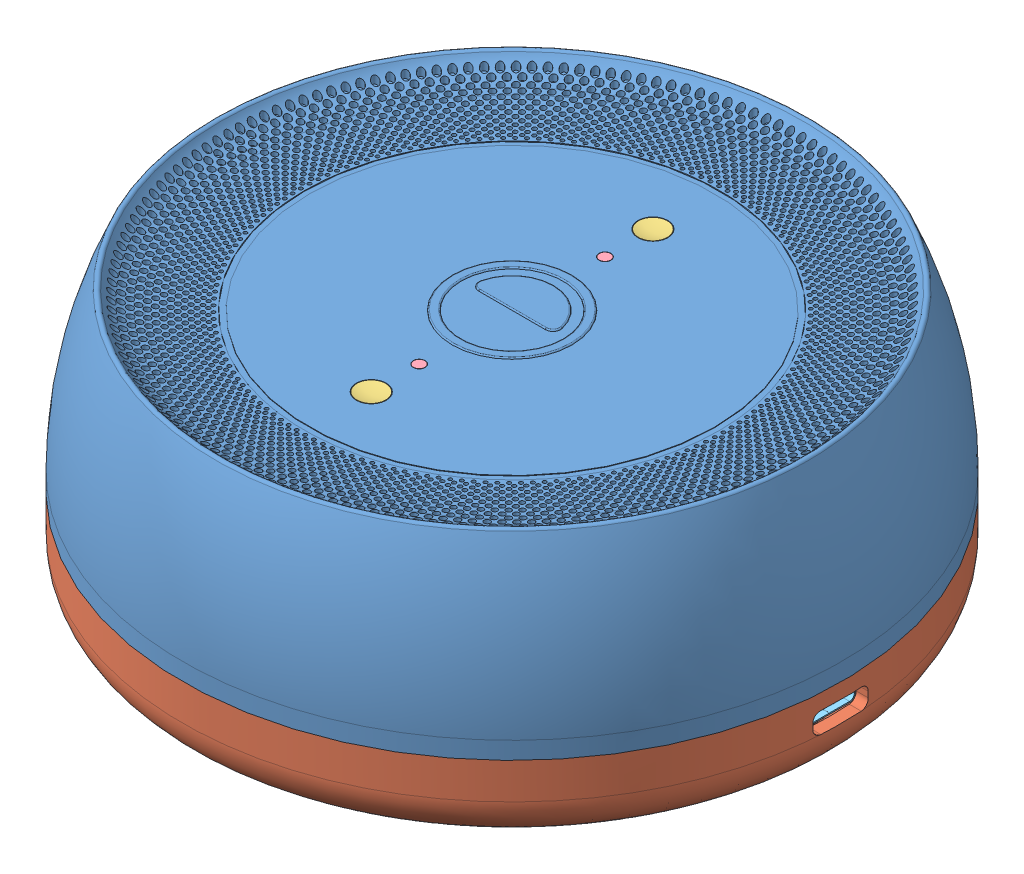
SolidWorks assembly Сборка, configuration Default. Lengths in mm.
Overall size (110 43.02 110).
434 component instances, 58 part files, 28 mates.
Components (placement in the parent):
- Корпус-1: Корпус [Default] at (55.5185 45.3642 75.701) size (110 29.48 110)
- Крышка-1: Крышка [Default] at (55.5185 43.2142 75.701) size (110 20.5 110)
- Кнопка-1: Кнопка [Default] at (55.5185 66.8642 99.201) size (7 2.5 7)
- Кнопка-2: Кнопка [Default] at (55.5185 66.8642 52.201) size (7 2.5 7)
- Держатель батареек-1: Держатель батареек [Default] at (94.5185 37.2764 95.701) x (0 0 -1) z (1 0 0) size (40 21.5 78)
- ME2CO-1: ME2CO [Default] at (52.3216 36.0894 105.6741) size (20 17 20)
- bottom_test_pcb-2: bottom_test_pcb [Default] at (55.5185 35.6764 75.701) x (1 0 0) z (0 -1 0) size (102.89 89.9 16)
  - USB Type C-1: USB Type C [По умолчанию] at origin size (11.79 8.75 4.86)
    - 632723300011-1: 632723300011 [По умолчанию] at (48.1249 -0.0001 -3.2614) x (0 1 0) z (1 0 0) size (8.75 4.86 11.79)
      - 632723300011_Shielding_2-1: 632723300011_Shielding_2 [По умолчанию] at (0 -0.8 -1.425) x (0 0 1) z (0 -1 0) size (2.92 7.5 1.07)
      - 632723300011_Shielding_2-2: 632723300011_Shielding_2 [По умолчанию] at (0 0.75 -1.425) x (0 0 1) z (0 1 0) size (2.92 7.5 1.07)
      - 632723300011_Housing_Bottom3-1: 632723300011_Housing_Bottom3 [По умолчанию] at (0 0.89 -5.284) x (-1 0 0) z (0 -1 0) size (6.46 2.1 0.78)
      - 632723300011_PIN7_Bottom_v3_mir-1: 632723300011_PIN7_Bottom_v3_mir [По умолчанию] at (0.4 3.3765 -5.46) x (-1 0 0) z (0 -1 0) size (0.54 7.67 3.25)
      - 632723300011_PIN5_Bottom_v3_mir-1: 632723300011_PIN5_Bottom_v3_mir [По умолчанию] at (1.2 3.3765 -5.46) x (-1 0 0) z (0 -1 0) size (0.37 8.17 3.21)
      - 632723300011_PIN2_Bottom_v3_mir-1: 632723300011_PIN2_Bottom_v3_mir [По умолчанию] at (2.4 3.3765 -4.75) x (-1 0 0) z (0 -1 0) size (0.54 6.96 3.25)
      - 632723300011_PIN6_Bottom_v3_mir-1: 632723300011_PIN6_Bottom_v3_mir [По умолчанию] at (0.8 3.3765 -4.76) x (-1 0 0) z (0 -1 0) size (0.4 6.97 3.21)
      - 632723300011_PIN4_Bottom_v3_mir-1: 632723300011_PIN4_Bottom_v3_mir [По умолчанию] at (1.6 3.3765 -4.7565) x (-1 0 0) z (0 -1 0) size (0.52 7.01 3.21)
      - 632723300011_PIN1_Bottom_v3_mir-1: 632723300011_PIN1_Bottom_v3_mir [По умолчанию] at (2.8 3.3765 -5.46) x (-1 0 0) z (0 -1 0) size (0.4 8.17 3.21)
      - 632723300011_PIN2_Top_v3-1: 632723300011_PIN2_Top_v3 [По умолчанию] at (1.75 2.37 -6.335) x (0 0 1) z (0 -1 0) size (9.09 0.28 1.93)
      - 632723300011_PIN2_Top_v3-2: 632723300011_PIN2_Top_v3 [По умолчанию] at (-1.75 2.37 -6.335) x (0 0 1) z (0 -1 0) size (9.09 0.28 1.93)
      - 632723300011_PIN2_Top_v3-3: 632723300011_PIN2_Top_v3 [По умолчанию] at (-0.75 2.37 -6.335) x (0 0 1) z (0 -1 0) size (9.09 0.28 1.93)
      - 632723300011_PIN2_Top_v3-4: 632723300011_PIN2_Top_v3 [По умолчанию] at (0.75 2.37 -6.335) x (0 0 1) z (0 -1 0) size (9.09 0.28 1.93)
      - 632723300011_PIN2_Top_v3-5: 632723300011_PIN2_Top_v3 [По умолчанию] at (-0.25 2.37 -6.335) x (0 0 1) z (0 -1 0) size (9.09 0.28 1.93)
      - 632723300011_PIN2_Top_v3-6: 632723300011_PIN2_Top_v3 [По умолчанию] at (2.25 2.37 -6.335) x (0 0 1) z (0 -1 0) size (9.09 0.28 1.93)
      - 632723300011_PIN2_Top_v3-7: 632723300011_PIN2_Top_v3 [По умолчанию] at (0.25 2.37 -6.335) x (0 0 1) z (0 -1 0) size (9.09 0.28 1.93)
      - 632723300011_PIN2_Top_v3-8: 632723300011_PIN2_Top_v3 [По умолчанию] at (-2.25 2.37 -6.335) x (0 0 1) z (0 -1 0) size (9.09 0.28 1.93)
      - 632723300011_PIN7_Bottom_v3-1: 632723300011_PIN7_Bottom_v3 [По умолчанию] at (-0.4 3.3765 -5.46) x (1 0 0) z (0 -1 0) size (0.54 7.67 3.21)
      - 632723300011_PIN6_Bottom_v3-1: 632723300011_PIN6_Bottom_v3 [По умолчанию] at (-0.8 3.3765 -4.76) x (1 0 0) z (0 -1 0) size (0.4 6.97 3.22)
      - 632723300011_PIN5_Bottom_v3-1: 632723300011_PIN5_Bottom_v3 [По умолчанию] at (-1.2 3.3765 -5.46) x (1 0 0) z (0 -1 0) size (0.37 8.17 3.19)
      - 632723300011_PIN4_Bottom_v3-1: 632723300011_PIN4_Bottom_v3 [По умолчанию] at (-1.6 3.3765 -4.7565) x (1 0 0) z (0 -1 0) size (0.54 7.01 3.25)
      - 632723300011_PIN2_Bottom_v3-1: 632723300011_PIN2_Bottom_v3 [По умолчанию] at (-2.4 3.3765 -4.75) x (1 0 0) z (0 -1 0) size (0.54 6.96 3.21)
      - 632723300011_PIN1_Top_v3-1: 632723300011_PIN1_Top_v3 [По умолчанию] at (2.75 1.97 -6.335) x (0 0 1) z (0 -1 0) size (9.59 0.28 1.93)
      - 632723300011_PIN1_Top_v3-2: 632723300011_PIN1_Top_v3 [По умолчанию] at (-1.25 1.97 -6.335) x (0 0 1) z (0 -1 0) size (9.59 0.28 1.93)
      - 632723300011_PIN1_Top_v3-3: 632723300011_PIN1_Top_v3 [По умолчанию] at (-2.75 1.97 -6.335) x (0 0 1) z (0 -1 0) size (9.59 0.28 1.93)
      - 632723300011_PIN1_Top_v3-4: 632723300011_PIN1_Top_v3 [По умолчанию] at (1.25 1.97 -6.335) x (0 0 1) z (0 -1 0) size (9.59 0.28 1.93)
      - 632723300011_PIN1_Bottom_v3-1: 632723300011_PIN1_Bottom_v3 [По умолчанию] at (-2.8 3.3765 -5.46) x (1 0 0) z (0 -1 0) size (0.4 8.17 3.22)
      - 632723300011_Housing_Bottom-1: 632723300011_Housing_Bottom [По умолчанию] at (0 0.89 -5.285) x (-1 0 0) z (0 -1 0) size (8.34 5.47 2.38)
      - 632723300011_Shielding_1_v3-1: 632723300011_Shielding_1_v3 [По умолчанию] at (0 0 -0.475) x (-1 0 0) z (0 -1 0) size (8.75 10.6 4.86)
      - 632723300011_Housing_TOP-1: 632723300011_Housing_TOP [По умолчанию] at (0 -0.6 -3.9) x (1 0 0) z (0 -1 0) size (6.7 3.25 1.23)
      - 632723300011_Shielding_3_v3-1: 632723300011_Shielding_3_v3 [По умолчанию] at (0 0.05 0) size (7.5 3.43 8.64)
      - 632723300011_Housing-1: 632723300011_Housing [По умолчанию] at origin size (8.34 2.56 8.2)
  - C1-1: C1 [По умолчанию] at origin size (1.8 3.4 1.8)
    - 6038255504-1: 6038255504 [По умолчанию] at (35.6 7.5 0) size (1.8 3.4 1.8)
      - Extruded-1: Extruded [По умолчанию] at origin size (1.8 3.4 1.8)
  - C2-1: C2 [По умолчанию] at origin size (1.45 2.2 1.55)
    - 6038248944-1: 6038248944 [По умолчанию] at (33 7.375 0) size (1.45 0.5 1.55)
      - Extruded-1-1: Extruded-1 [По умолчанию] at origin size (1.45 0.5 1.55)
    - 6038248944-2: 6038248944 [По умолчанию] at (33 5.675 0) size (1.45 0.5 1.55)
      - Extruded-1-1: Extruded-1 [По умолчанию] at origin size (1.45 0.5 1.55)
    - 6038249184-1: 6038249184 [По умолчанию] at (33 6.525 0) size (1.45 1.2 1.55)
      - Extruded-2-1: Extruded-2 [По умолчанию] at origin size (1.45 1.2 1.55)
  - C3-1: C3 [По умолчанию] at origin size (2.2 1.45 1.55)
    - 6038256064-1: 6038256064 [По умолчанию] at (30.15 2.5 0) size (0.5 1.45 1.55)
      - Extruded-3-1: Extruded-3 [По умолчанию] at origin size (0.5 1.45 1.55)
    - 6038256064-2: 6038256064 [По умолчанию] at (28.45 2.5 0) size (0.5 1.45 1.55)
      - Extruded-3-1: Extruded-3 [По умолчанию] at origin size (0.5 1.45 1.55)
    - 6038256544-1: 6038256544 [По умолчанию] at (29.3 2.5 0) size (1.2 1.45 1.55)
      - Extruded-4-1: Extruded-4 [По умолчанию] at origin size (1.2 1.45 1.55)
  - C4-1: C4 [По умолчанию] at origin size (2.2 1.45 1.55)
    - 6038256064-1: 6038256064 [По умолчанию] at (31.95 9.3 0) size (0.5 1.45 1.55)
      - Extruded-3-1: Extruded-3 [По умолчанию] at origin size (0.5 1.45 1.55)
    - 6038256064-2: 6038256064 [По умолчанию] at (30.25 9.3 0) size (0.5 1.45 1.55)
      - Extruded-3-1: Extruded-3 [По умолчанию] at origin size (0.5 1.45 1.55)
    - 6038256544-1: 6038256544 [По умолчанию] at (31.1 9.3 0) size (1.2 1.45 1.55)
      - Extruded-4-1: Extruded-4 [По умолчанию] at origin size (1.2 1.45 1.55)
  - C5-1: C5 [По умолчанию] at origin size (1.8 3.4 1.8)
    - 6038255504-1: 6038255504 [По умолчанию] at (36.9 15.75 0) size (1.8 3.4 1.8)
      - Extruded-1: Extruded [По умолчанию] at origin size (1.8 3.4 1.8)
  - C6-1: C6 [По умолчанию] at origin size (1.45 2.2 1.55)
    - 6038248944-1: 6038248944 [По умолчанию] at (-24.655 -38.95 0) size (1.45 0.5 1.55)
      - Extruded-1-1: Extruded-1 [По умолчанию] at origin size (1.45 0.5 1.55)
    - 6038248944-2: 6038248944 [По умолчанию] at (-24.655 -37.25 0) size (1.45 0.5 1.55)
      - Extruded-1-1: Extruded-1 [По умолчанию] at origin size (1.45 0.5 1.55)
    - 6038249184-1: 6038249184 [По умолчанию] at (-24.655 -38.1 0) size (1.45 1.2 1.55)
      - Extruded-2-1: Extruded-2 [По умолчанию] at origin size (1.45 1.2 1.55)
  - C7-1: C7 [По умолчанию] at origin size (2.2 1.45 1.55)
    - 6038256064-1: 6038256064 [По умолчанию] at (32.8 28.7 0) size (0.5 1.45 1.55)
      - Extruded-3-1: Extruded-3 [По умолчанию] at origin size (0.5 1.45 1.55)
    - 6038256064-2: 6038256064 [По умолчанию] at (34.5 28.7 0) size (0.5 1.45 1.55)
      - Extruded-3-1: Extruded-3 [По умолчанию] at origin size (0.5 1.45 1.55)
    - 6038256544-1: 6038256544 [По умолчанию] at (33.65 28.7 0) size (1.2 1.45 1.55)
      - Extruded-4-1: Extruded-4 [По умолчанию] at origin size (1.2 1.45 1.55)
  - C8-1: C8 [По умолчанию] at origin size (1.45 2.2 1.55)
    - 6038248944-1: 6038248944 [По умолчанию] at (14.5249 -39.225 0) size (1.45 0.5 1.55)
      - Extruded-1-1: Extruded-1 [По умолчанию] at origin size (1.45 0.5 1.55)
    - 6038248944-2: 6038248944 [По умолчанию] at (14.5249 -40.925 0) size (1.45 0.5 1.55)
      - Extruded-1-1: Extruded-1 [По умолчанию] at origin size (1.45 0.5 1.55)
    - 6038249184-1: 6038249184 [По умолчанию] at (14.5249 -40.075 0) size (1.45 1.2 1.55)
      - Extruded-2-1: Extruded-2 [По умолчанию] at origin size (1.45 1.2 1.55)
  - C9-1: C9 [По умолчанию] at origin size (1.45 2.2 1.55)
    - 6038248944-1: 6038248944 [По умолчанию] at (12.5999 -39.225 0) size (1.45 0.5 1.55)
      - Extruded-1-1: Extruded-1 [По умолчанию] at origin size (1.45 0.5 1.55)
    - 6038248944-2: 6038248944 [По умолчанию] at (12.5999 -40.925 0) size (1.45 0.5 1.55)
      - Extruded-1-1: Extruded-1 [По умолчанию] at origin size (1.45 0.5 1.55)
    - 6038249184-1: 6038249184 [По умолчанию] at (12.5999 -40.075 0) size (1.45 1.2 1.55)
      - Extruded-2-1: Extruded-2 [По умолчанию] at origin size (1.45 1.2 1.55)
  - C10-1: C10 [По умолчанию] at origin size (1.45 2.2 1.55)
    - 6038248944-1: 6038248944 [По умолчанию] at (10.6499 -39.215 0) size (1.45 0.5 1.55)
      - Extruded-1-1: Extruded-1 [По умолчанию] at origin size (1.45 0.5 1.55)
    - 6038248944-2: 6038248944 [По умолчанию] at (10.6499 -40.915 0) size (1.45 0.5 1.55)
      - Extruded-1-1: Extruded-1 [По умолчанию] at origin size (1.45 0.5 1.55)
    - 6038249184-1: 6038249184 [По умолчанию] at (10.6499 -40.065 0) size (1.45 1.2 1.55)
      - Extruded-2-1: Extruded-2 [По умолчанию] at origin size (1.45 1.2 1.55)
  - C11-1: C11 [По умолчанию] at origin size (1.8 3.4 1.8)
    - 6038255504-1: 6038255504 [По умолчанию] at (17.0249 -39.575 0) size (1.8 3.4 1.8)
      - Extruded-1: Extruded [По умолчанию] at origin size (1.8 3.4 1.8)
  - C12-1: C12 [По умолчанию] at origin size (2.2 1.45 1.55)
    - 6038256064-1: 6038256064 [По умолчанию] at (1.85 -14 0) size (0.5 1.45 1.55)
      - Extruded-3-1: Extruded-3 [По умолчанию] at origin size (0.5 1.45 1.55)
    - 6038256064-2: 6038256064 [По умолчанию] at (0.15 -14 0) size (0.5 1.45 1.55)
      - Extruded-3-1: Extruded-3 [По умолчанию] at origin size (0.5 1.45 1.55)
    - 6038256544-1: 6038256544 [По умолчанию] at (1 -14 0) size (1.2 1.45 1.55)
      - Extruded-4-1: Extruded-4 [По умолчанию] at origin size (1.2 1.45 1.55)
  - C13-1: C13 [По умолчанию] at origin size (3.4 1.8 1.8)
    - 6038245584-1: 6038245584 [По умолчанию] at (-16.405 -38.725 0) size (3.4 1.8 1.8)
      - Extruded-5-1: Extruded-5 [По умолчанию] at origin size (3.4 1.8 1.8)
  - C14-1: C14 [По умолчанию] at origin size (1.45 2.2 1.55)
    - 6038248944-1: 6038248944 [По умолчанию] at (23.1 13.8 0) size (1.45 0.5 1.55)
      - Extruded-1-1: Extruded-1 [По умолчанию] at origin size (1.45 0.5 1.55)
    - 6038248944-2: 6038248944 [По умолчанию] at (23.1 15.5 0) size (1.45 0.5 1.55)
      - Extruded-1-1: Extruded-1 [По умолчанию] at origin size (1.45 0.5 1.55)
    - 6038249184-1: 6038249184 [По умолчанию] at (23.1 14.65 0) size (1.45 1.2 1.55)
      - Extruded-2-1: Extruded-2 [По умолчанию] at origin size (1.45 1.2 1.55)
  - C15-1: C15 [По умолчанию] at origin size (2.2 1.45 1.55)
    - 6038256064-1: 6038256064 [По умолчанию] at (5.15 22.15 0) size (0.5 1.45 1.55)
      - Extruded-3-1: Extruded-3 [По умолчанию] at origin size (0.5 1.45 1.55)
    - 6038256064-2: 6038256064 [По умолчанию] at (3.45 22.15 0) size (0.5 1.45 1.55)
      - Extruded-3-1: Extruded-3 [По умолчанию] at origin size (0.5 1.45 1.55)
    - 6038256544-1: 6038256544 [По умолчанию] at (4.3 22.15 0) size (1.2 1.45 1.55)
      - Extruded-4-1: Extruded-4 [По умолчанию] at origin size (1.2 1.45 1.55)
  - C16-1: C16 [По умолчанию] at origin size (1.45 2.2 1.55)
    - 6038248944-1: 6038248944 [По умолчанию] at (-3.2 25.85 0) size (1.45 0.5 1.55)
      - Extruded-1-1: Extruded-1 [По умолчанию] at origin size (1.45 0.5 1.55)
    - 6038248944-2: 6038248944 [По умолчанию] at (-3.2 24.15 0) size (1.45 0.5 1.55)
      - Extruded-1-1: Extruded-1 [По умолчанию] at origin size (1.45 0.5 1.55)
    - 6038249184-1: 6038249184 [По умолчанию] at (-3.2 25 0) size (1.45 1.2 1.55)
      - Extruded-2-1: Extruded-2 [По умолчанию] at origin size (1.45 1.2 1.55)
  - C17-1: C17 [По умолчанию] at origin size (3.4 1.8 1.8)
    - 6038245584-1: 6038245584 [По умолчанию] at (-1.45 13.375 0) size (3.4 1.8 1.8)
      - Extruded-5-1: Extruded-5 [По умолчанию] at origin size (3.4 1.8 1.8)
  - C18-1: C18 [По умолчанию] at origin size (1.45 2.2 1.55)
    - 6038248944-1: 6038248944 [По умолчанию] at (-2.15 8.35 0) size (1.45 0.5 1.55)
      - Extruded-1-1: Extruded-1 [По умолчанию] at origin size (1.45 0.5 1.55)
    - 6038248944-2: 6038248944 [По умолчанию] at (-2.15 10.05 0) size (1.45 0.5 1.55)
      - Extruded-1-1: Extruded-1 [По умолчанию] at origin size (1.45 0.5 1.55)
    - 6038249184-1: 6038249184 [По умолчанию] at (-2.15 9.2 0) size (1.45 1.2 1.55)
      - Extruded-2-1: Extruded-2 [По умолчанию] at origin size (1.45 1.2 1.55)
  - C19-1: C19 [По умолчанию] at origin size (3.4 1.8 1.8)
    - 6038245584-1: 6038245584 [По умолчанию] at (-3.775 3.325 0) size (3.4 1.8 1.8)
      - Extruded-5-1: Extruded-5 [По умолчанию] at origin size (3.4 1.8 1.8)
  - C20-1: C20 [По умолчанию] at origin size (2.2 1.45 1.55)
    - 6038256064-1: 6038256064 [По умолчанию] at (-5.125 5.975 0) size (0.5 1.45 1.55)
      - Extruded-3-1: Extruded-3 [По умолчанию] at origin size (0.5 1.45 1.55)
    - 6038256064-2: 6038256064 [По умолчанию] at (-3.425 5.975 0) size (0.5 1.45 1.55)
      - Extruded-3-1: Extruded-3 [По умолчанию] at origin size (0.5 1.45 1.55)
    - 6038256544-1: 6038256544 [По умолчанию] at (-4.275 5.975 0) size (1.2 1.45 1.55)
      - Extruded-4-1: Extruded-4 [По умолчанию] at origin size (1.2 1.45 1.55)
  - C21-1: C21 [По умолчанию] at origin size (1.45 2.2 1.55)
    - 6038248944-1: 6038248944 [По умолчанию] at (-33.19 -13.785 0) size (1.45 0.5 1.55)
      - Extruded-1-1: Extruded-1 [По умолчанию] at origin size (1.45 0.5 1.55)
    - 6038248944-2: 6038248944 [По умолчанию] at (-33.19 -12.085 0) size (1.45 0.5 1.55)
      - Extruded-1-1: Extruded-1 [По умолчанию] at origin size (1.45 0.5 1.55)
    - 6038249184-1: 6038249184 [По умолчанию] at (-33.19 -12.935 0) size (1.45 1.2 1.55)
      - Extruded-2-1: Extruded-2 [По умолчанию] at origin size (1.45 1.2 1.55)
  - C22-1: C22 [По умолчанию] at origin size (1.45 2.2 1.55)
    - 6038248944-1: 6038248944 [По умолчанию] at (-33.14 -15.41 0) size (1.45 0.5 1.55)
      - Extruded-1-1: Extruded-1 [По умолчанию] at origin size (1.45 0.5 1.55)
    - 6038248944-2: 6038248944 [По умолчанию] at (-33.14 -17.11 0) size (1.45 0.5 1.55)
      - Extruded-1-1: Extruded-1 [По умолчанию] at origin size (1.45 0.5 1.55)
    - 6038249184-1: 6038249184 [По умолчанию] at (-33.14 -16.26 0) size (1.45 1.2 1.55)
      - Extruded-2-1: Extruded-2 [По умолчанию] at origin size (1.45 1.2 1.55)
  - DA1-1: DA1 [По умолчанию] at origin size (3 3 1)
    - 6039004688-1: 6039004688 [По умолчанию] at (29.5 5.5 0) size (3 3 1)
      - Extruded-6-1: Extruded-6 [По умолчанию] at origin size (3 3 1)
  - DA2-1: DA2 [По умолчанию] at origin size (2.59 4.6 1.6)
    - 6039009248-1: 6039009248 [По умолчанию] at (29 24.7 0) size (2.59 4.6 1.6)
      - Extruded-7-1: Extruded-7 [По умолчанию] at origin size (2.59 4.6 1.6)
  - DA3-1: DA3 [По умолчанию] at origin size (2.59 4.6 1.6)
    - 6039009248-1: 6039009248 [По умолчанию] at (29.705 -13 0) size (2.59 4.6 1.6)
      - Extruded-7-1: Extruded-7 [По умолчанию] at origin size (2.59 4.6 1.6)
  - DA4-1: DA4 [По умолчанию] at origin size (1.6 2.9 1)
    - 6038242784-1: 6038242784 [По умолчанию] at (6.35 25.175 0) size (1.6 2.9 1)
      - Extruded-8-1: Extruded-8 [По умолчанию] at origin size (1.6 2.9 1)
  - DA5-1: DA5 [По умолчанию] at origin size (1.6 2.9 1)
    - 6038242784-1: 6038242784 [По умолчанию] at (0.075 25.15 0) size (1.6 2.9 1)
      - Extruded-8-1: Extruded-8 [По умолчанию] at origin size (1.6 2.9 1)
  - DD1-1: DD1 [По умолчанию] at origin size (18.07 25.54 3.04)
    - User Library-esp-wroom-32-1: User Library-esp-wroom-32 [По умолчанию] at (8.5751 -22.0099 0.035) x (-1 0 0) z (0 1 0) size (18.07 3.04 25.54)
  - DD2-1: DD2 [По умолчанию] at origin size (3.1 1.8 1.45)
    - 6038246384-1: 6038246384 [По умолчанию] at (-5.075 9.225 0) size (3.1 1.8 1.45)
      - Extruded-9-1: Extruded-9 [По умолчанию] at origin size (3.1 1.8 1.45)
  - LS1-1: LS1 [По умолчанию] at origin size (12 12 16)
    - 6038997088-1: 6038997088 [По умолчанию] at (-29.9999 -31.25 5.8086) x (0 1 0) z (0 0 -1) size (0.6 0.6 7.5)
      - Cylinder-1: Cylinder [По умолчанию] at origin size (0.6 0.6 7.5)
    - 6038997488-1: 6038997488 [По умолчанию] at (-30 -24.7499 3.8086) x (0 1 0) z (0 0 -1) size (0.6 0.6 5.5)
      - Cylinder-1-1: Cylinder-1 [По умолчанию] at origin size (0.6 0.6 5.5)
    - 6038996448-1: 6038996448 [По умолчанию] at (-30 -28 -9.6914) size (2.3 2.3 4.7)
      - Extruded-10-1: Extruded-10 [По умолчанию] at origin size (2.3 2.3 4.7)
    - 6038996528-1: 6038996528 [По умолчанию] at (-30 -28 -4.6914) size (12 12 3)
      - Extruded-11-1: Extruded-11 [По умолчанию] at origin size (12 12 3)
    - 6038996608-1: 6038996608 [По умолчанию] at (-30 -28 -4.9914) size (10 10 0.3)
      - Extruded-12-1: Extruded-12 [По умолчанию] at origin size (10 10 0.3)
    - 6038996368-1: 6038996368 [По умолчанию] at (-30 -28 -10.1914) size (12 12 5.2)
  - R1-1: R1 [По умолчанию] at origin size (1.35 2.2 0.7)
    - 6038252864-1: 6038252864 [По умолчанию] at (35.1 -3.24 0) size (1.35 0.42 0.7)
      - Extruded-13-1: Extruded-13 [По умолчанию] at origin size (1.35 0.42 0.7)
    - 6038252544-1: 6038252544 [По умолчанию] at (35.1 -2.35 0) size (1.35 1.36 0.7)
      - Extruded-14-1: Extruded-14 [По умолчанию] at origin size (1.35 1.36 0.7)
    - 6038252864-2: 6038252864 [По умолчанию] at (35.1 -1.46 0) size (1.35 0.42 0.7)
      - Extruded-13-1: Extruded-13 [По умолчанию] at origin size (1.35 0.42 0.7)
  - R2-1: R2 [По умолчанию] at origin size (1.35 2.2 0.7)
    - 6038252864-1: 6038252864 [По умолчанию] at (32.5 -5.44 0) size (1.35 0.42 0.7)
      - Extruded-13-1: Extruded-13 [По умолчанию] at origin size (1.35 0.42 0.7)
    - 6038252544-1: 6038252544 [По умолчанию] at (32.5 -4.55 0) size (1.35 1.36 0.7)
      - Extruded-14-1: Extruded-14 [По умолчанию] at origin size (1.35 1.36 0.7)
    - 6038252864-2: 6038252864 [По умолчанию] at (32.5 -3.66 0) size (1.35 0.42 0.7)
      - Extruded-13-1: Extruded-13 [По умолчанию] at origin size (1.35 0.42 0.7)
  - R3-1: R3 [По умолчанию] at origin size (1.35 2.2 0.7)
    - 6038252864-1: 6038252864 [По умолчанию] at (27.3 -5.49 0) size (1.35 0.42 0.7)
      - Extruded-13-1: Extruded-13 [По умолчанию] at origin size (1.35 0.42 0.7)
    - 6038252544-1: 6038252544 [По умолчанию] at (27.3 -4.6 0) size (1.35 1.36 0.7)
      - Extruded-14-1: Extruded-14 [По умолчанию] at origin size (1.35 1.36 0.7)
    - 6038252864-2: 6038252864 [По умолчанию] at (27.3 -3.71 0) size (1.35 0.42 0.7)
      - Extruded-13-1: Extruded-13 [По умолчанию] at origin size (1.35 0.42 0.7)
  - R4-1: R4 [По умолчанию] at origin size (1.35 2.2 0.7)
    - 6038252864-1: 6038252864 [По умолчанию] at (29.9 -5.49 0) size (1.35 0.42 0.7)
      - Extruded-13-1: Extruded-13 [По умолчанию] at origin size (1.35 0.42 0.7)
    - 6038252544-1: 6038252544 [По умолчанию] at (29.9 -4.6 0) size (1.35 1.36 0.7)
      - Extruded-14-1: Extruded-14 [По умолчанию] at origin size (1.35 1.36 0.7)
    - 6038252864-2: 6038252864 [По умолчанию] at (29.9 -3.71 0) size (1.35 0.42 0.7)
      - Extruded-13-1: Extruded-13 [По умолчанию] at origin size (1.35 0.42 0.7)
  - R5-1: R5 [По умолчанию] at origin size (2.2 1.35 0.7)
    - 6038254144-1: 6038254144 [По умолчанию] at (28.19 -0.9 0) size (0.42 1.35 0.7)
      - Extruded-15-1: Extruded-15 [По умолчанию] at origin size (0.42 1.35 0.7)
    - 6038253744-1: 6038253744 [По умолчанию] at (27.3 -0.9 0) size (1.36 1.35 0.7)
      - Extruded-16-1: Extruded-16 [По умолчанию] at origin size (1.36 1.35 0.7)
    - 6038254144-2: 6038254144 [По умолчанию] at (26.41 -0.9 0) size (0.42 1.35 0.7)
      - Extruded-15-1: Extruded-15 [По умолчанию] at origin size (0.42 1.35 0.7)
  - R6-1: R6 [По умолчанию] at origin size (2.2 1.35 0.7)
    - 6038254144-1: 6038254144 [По умолчанию] at (13.1599 -13.675 0) size (0.42 1.35 0.7)
      - Extruded-15-1: Extruded-15 [По умолчанию] at origin size (0.42 1.35 0.7)
    - 6038253744-1: 6038253744 [По умолчанию] at (14.0499 -13.675 0) size (1.36 1.35 0.7)
      - Extruded-16-1: Extruded-16 [По умолчанию] at origin size (1.36 1.35 0.7)
    - 6038254144-2: 6038254144 [По умолчанию] at (14.9399 -13.675 0) size (0.42 1.35 0.7)
      - Extruded-15-1: Extruded-15 [По умолчанию] at origin size (0.42 1.35 0.7)
  - R7-1: R7 [По умолчанию] at origin size (2.2 1.35 0.7)
    - 6038254144-1: 6038254144 [По умолчанию] at (13.1599 -16.375 0) size (0.42 1.35 0.7)
      - Extruded-15-1: Extruded-15 [По умолчанию] at origin size (0.42 1.35 0.7)
    - 6038253744-1: 6038253744 [По умолчанию] at (14.05 -16.375 0) size (1.36 1.35 0.7)
      - Extruded-16-1: Extruded-16 [По умолчанию] at origin size (1.36 1.35 0.7)
    - 6038254144-2: 6038254144 [По умолчанию] at (14.9399 -16.375 0) size (0.42 1.35 0.7)
      - Extruded-15-1: Extruded-15 [По умолчанию] at origin size (0.42 1.35 0.7)
  - R8-1: R8 [По умолчанию] at origin size (2.2 1.35 0.7)
    - 6038254144-1: 6038254144 [По умолчанию] at (13.16 -21.675 0) size (0.42 1.35 0.7)
      - Extruded-15-1: Extruded-15 [По умолчанию] at origin size (0.42 1.35 0.7)
    - 6038253744-1: 6038253744 [По умолчанию] at (14.05 -21.675 0) size (1.36 1.35 0.7)
      - Extruded-16-1: Extruded-16 [По умолчанию] at origin size (1.36 1.35 0.7)
    - 6038254144-2: 6038254144 [По умолчанию] at (14.94 -21.675 0) size (0.42 1.35 0.7)
      - Extruded-15-1: Extruded-15 [По умолчанию] at origin size (0.42 1.35 0.7)
  - R9-1: R9 [По умолчанию] at origin size (2.2 1.35 0.7)
    - 6038254144-1: 6038254144 [По умолчанию] at (14.94 -19.025 0) size (0.42 1.35 0.7)
      - Extruded-15-1: Extruded-15 [По умолчанию] at origin size (0.42 1.35 0.7)
    - 6038253744-1: 6038253744 [По умолчанию] at (14.05 -19.025 0) size (1.36 1.35 0.7)
      - Extruded-16-1: Extruded-16 [По умолчанию] at origin size (1.36 1.35 0.7)
    - 6038254144-2: 6038254144 [По умолчанию] at (13.16 -19.025 0) size (0.42 1.35 0.7)
      - Extruded-15-1: Extruded-15 [По умолчанию] at origin size (0.42 1.35 0.7)
  - R10-1: R10 [По умолчанию] at origin size (2.2 1.35 0.7)
    - 6038254144-1: 6038254144 [По умолчанию] at (-12.84 -23.5 0) size (0.42 1.35 0.7)
      - Extruded-15-1: Extruded-15 [По умолчанию] at origin size (0.42 1.35 0.7)
    - 6038253744-1: 6038253744 [По умолчанию] at (-13.73 -23.5 0) size (1.36 1.35 0.7)
      - Extruded-16-1: Extruded-16 [По умолчанию] at origin size (1.36 1.35 0.7)
    - 6038254144-2: 6038254144 [По умолчанию] at (-14.62 -23.5 0) size (0.42 1.35 0.7)
      - Extruded-15-1: Extruded-15 [По умолчанию] at origin size (0.42 1.35 0.7)
  - R11-1: R11 [По умолчанию] at origin size (2.2 1.35 0.7)
    - 6038254144-1: 6038254144 [По умолчанию] at (-15.815 -32.925 0) size (0.42 1.35 0.7)
      - Extruded-15-1: Extruded-15 [По умолчанию] at origin size (0.42 1.35 0.7)
    - 6038253744-1: 6038253744 [По умолчанию] at (-16.705 -32.925 0) size (1.36 1.35 0.7)
      - Extruded-16-1: Extruded-16 [По умолчанию] at origin size (1.36 1.35 0.7)
    - 6038254144-2: 6038254144 [По умолчанию] at (-17.595 -32.925 0) size (0.42 1.35 0.7)
      - Extruded-15-1: Extruded-15 [По умолчанию] at origin size (0.42 1.35 0.7)
  - R12-1: R12 [По умолчанию] at origin size (2.2 1.35 0.7)
    - 6038254144-1: 6038254144 [По умолчанию] at (-15.79 -35.675 0) size (0.42 1.35 0.7)
      - Extruded-15-1: Extruded-15 [По умолчанию] at origin size (0.42 1.35 0.7)
    - 6038253744-1: 6038253744 [По умолчанию] at (-16.68 -35.675 0) size (1.36 1.35 0.7)
      - Extruded-16-1: Extruded-16 [По умолчанию] at origin size (1.36 1.35 0.7)
    - 6038254144-2: 6038254144 [По умолчанию] at (-17.57 -35.675 0) size (0.42 1.35 0.7)
      - Extruded-15-1: Extruded-15 [По умолчанию] at origin size (0.42 1.35 0.7)
  - R13-1: R13 [По умолчанию] at origin size (2.2 1.35 0.7)
    - 6038254144-1: 6038254144 [По умолчанию] at (-16.58 -16.385 0) size (0.42 1.35 0.7)
      - Extruded-15-1: Extruded-15 [По умолчанию] at origin size (0.42 1.35 0.7)
    - 6038253744-1: 6038253744 [По умолчанию] at (-15.69 -16.385 0) size (1.36 1.35 0.7)
      - Extruded-16-1: Extruded-16 [По умолчанию] at origin size (1.36 1.35 0.7)
    - 6038254144-2: 6038254144 [По умолчанию] at (-14.8 -16.385 0) size (0.42 1.35 0.7)
      - Extruded-15-1: Extruded-15 [По умолчанию] at origin size (0.42 1.35 0.7)
  - R14-1: R14 [По умолчанию] at origin size (1.35 2.2 0.7)
    - 6038252864-1: 6038252864 [По умолчанию] at (-21.29 -15.925 0) size (1.35 0.42 0.7)
      - Extruded-13-1: Extruded-13 [По умолчанию] at origin size (1.35 0.42 0.7)
    - 6038252544-1: 6038252544 [По умолчанию] at (-21.29 -15.035 0) size (1.35 1.36 0.7)
      - Extruded-14-1: Extruded-14 [По умолчанию] at origin size (1.35 1.36 0.7)
    - 6038252864-2: 6038252864 [По умолчанию] at (-21.29 -14.145 0) size (1.35 0.42 0.7)
      - Extruded-13-1: Extruded-13 [По умолчанию] at origin size (1.35 0.42 0.7)
  - R17-1: R17 [По умолчанию] at origin size (2.2 1.35 0.7)
    - 6038254144-1: 6038254144 [По умолчанию] at (14.94 -27 0) size (0.42 1.35 0.7)
      - Extruded-15-1: Extruded-15 [По умолчанию] at origin size (0.42 1.35 0.7)
    - 6038253744-1: 6038253744 [По умолчанию] at (14.05 -27 0) size (1.36 1.35 0.7)
      - Extruded-16-1: Extruded-16 [По умолчанию] at origin size (1.36 1.35 0.7)
    - 6038254144-2: 6038254144 [По умолчанию] at (13.16 -27 0) size (0.42 1.35 0.7)
      - Extruded-15-1: Extruded-15 [По умолчанию] at origin size (0.42 1.35 0.7)
  - R18-1: R18 [По умолчанию] at origin size (2.2 1.35 0.7)
    - 6038254144-1: 6038254144 [По умолчанию] at (14.94 -24.325 0) size (0.42 1.35 0.7)
      - Extruded-15-1: Extruded-15 [По умолчанию] at origin size (0.42 1.35 0.7)
    - 6038253744-1: 6038253744 [По умолчанию] at (14.05 -24.325 0) size (1.36 1.35 0.7)
      - Extruded-16-1: Extruded-16 [По умолчанию] at origin size (1.36 1.35 0.7)
    - 6038254144-2: 6038254144 [По умолчанию] at (13.16 -24.325 0) size (0.42 1.35 0.7)
      - Extruded-15-1: Extruded-15 [По умолчанию] at origin size (0.42 1.35 0.7)
  - R19-1: R19 [По умолчанию] at origin size (1.35 2.2 0.7)
    - 6038252864-1: 6038252864 [По умолчанию] at (7.65 21.54 0) size (1.35 0.42 0.7)
      - Extruded-13-1: Extruded-13 [По умолчанию] at origin size (1.35 0.42 0.7)
    - 6038252544-1: 6038252544 [По умолчанию] at (7.65 20.65 0) size (1.35 1.36 0.7)
      - Extruded-14-1: Extruded-14 [По умолчанию] at origin size (1.35 1.36 0.7)
    - 6038252864-2: 6038252864 [По умолчанию] at (7.65 19.76 0) size (1.35 0.42 0.7)
      - Extruded-13-1: Extruded-13 [По умолчанию] at origin size (1.35 0.42 0.7)
  - R20-1: R20 [По умолчанию] at origin size (2.2 1.35 0.7)
    - 6038254144-1: 6038254144 [По умолчанию] at (4.94 19.575 0) size (0.42 1.35 0.7)
      - Extruded-15-1: Extruded-15 [По умолчанию] at origin size (0.42 1.35 0.7)
    - 6038253744-1: 6038253744 [По умолчанию] at (4.05 19.575 0) size (1.36 1.35 0.7)
      - Extruded-16-1: Extruded-16 [По умолчанию] at origin size (1.36 1.35 0.7)
    - 6038254144-2: 6038254144 [По умолчанию] at (3.16 19.575 0) size (0.42 1.35 0.7)
      - Extruded-15-1: Extruded-15 [По умолчанию] at origin size (0.42 1.35 0.7)
  - R21-1: R21 [По умолчанию] at origin size (2.2 1.35 0.7)
    - 6038254144-1: 6038254144 [По умолчанию] at (-0.89 29.5 0) size (0.42 1.35 0.7)
      - Extruded-15-1: Extruded-15 [По умолчанию] at origin size (0.42 1.35 0.7)
    - 6038253744-1: 6038253744 [По умолчанию] at (0 29.5 0) size (1.36 1.35 0.7)
      - Extruded-16-1: Extruded-16 [По умолчанию] at origin size (1.36 1.35 0.7)
    - 6038254144-2: 6038254144 [По умолчанию] at (0.89 29.5 0) size (0.42 1.35 0.7)
      - Extruded-15-1: Extruded-15 [По умолчанию] at origin size (0.42 1.35 0.7)
  - R22-1: R22 [По умолчанию] at origin size (2.2 1.35 0.7)
    - 6038254144-1: 6038254144 [По умолчанию] at (-4.085 21.775 0) size (0.42 1.35 0.7)
      - Extruded-15-1: Extruded-15 [По умолчанию] at origin size (0.42 1.35 0.7)
    - 6038253744-1: 6038253744 [По умолчанию] at (-4.975 21.775 0) size (1.36 1.35 0.7)
      - Extruded-16-1: Extruded-16 [По умолчанию] at origin size (1.36 1.35 0.7)
    - 6038254144-2: 6038254144 [По умолчанию] at (-5.865 21.775 0) size (0.42 1.35 0.7)
      - Extruded-15-1: Extruded-15 [По умолчанию] at origin size (0.42 1.35 0.7)
  - R23-1: R23 [По умолчанию] at origin size (2.2 1.35 0.7)
    - 6038254144-1: 6038254144 [По умолчанию] at (0.49 21.75 0) size (0.42 1.35 0.7)
      - Extruded-15-1: Extruded-15 [По умолчанию] at origin size (0.42 1.35 0.7)
    - 6038253744-1: 6038253744 [По умолчанию] at (-0.4 21.75 0) size (1.36 1.35 0.7)
      - Extruded-16-1: Extruded-16 [По умолчанию] at origin size (1.36 1.35 0.7)
    - 6038254144-2: 6038254144 [По умолчанию] at (-1.29 21.75 0) size (0.42 1.35 0.7)
      - Extruded-15-1: Extruded-15 [По умолчанию] at origin size (0.42 1.35 0.7)
  - R24-1: R24 [По умолчанию] at origin size (2.2 1.35 0.7)
    - 6038254144-1: 6038254144 [По умолчанию] at (-1.29 16.475 0) size (0.42 1.35 0.7)
      - Extruded-15-1: Extruded-15 [По умолчанию] at origin size (0.42 1.35 0.7)
    - 6038253744-1: 6038253744 [По умолчанию] at (-0.4 16.475 0) size (1.36 1.35 0.7)
      - Extruded-16-1: Extruded-16 [По умолчанию] at origin size (1.36 1.35 0.7)
    - 6038254144-2: 6038254144 [По умолчанию] at (0.49 16.475 0) size (0.42 1.35 0.7)
      - Extruded-15-1: Extruded-15 [По умолчанию] at origin size (0.42 1.35 0.7)
  - R25-1: R25 [По умолчанию] at origin size (2.2 1.35 0.7)
    - 6038254144-1: 6038254144 [По умолчанию] at (-12.84 -26.075 0) size (0.42 1.35 0.7)
      - Extruded-15-1: Extruded-15 [По умолчанию] at origin size (0.42 1.35 0.7)
    - 6038253744-1: 6038253744 [По умолчанию] at (-13.73 -26.075 0) size (1.36 1.35 0.7)
      - Extruded-16-1: Extruded-16 [По умолчанию] at origin size (1.36 1.35 0.7)
    - 6038254144-2: 6038254144 [По умолчанию] at (-14.62 -26.075 0) size (0.42 1.35 0.7)
      - Extruded-15-1: Extruded-15 [По умолчанию] at origin size (0.42 1.35 0.7)
  - R26-1: R26 [По умолчанию] at origin size (2.2 1.35 0.7)
    - 6038254144-1: 6038254144 [По умолчанию] at (13.16 -29.675 0) size (0.42 1.35 0.7)
      - Extruded-15-1: Extruded-15 [По умолчанию] at origin size (0.42 1.35 0.7)
    - 6038253744-1: 6038253744 [По умолчанию] at (14.05 -29.675 0) size (1.36 1.35 0.7)
      - Extruded-16-1: Extruded-16 [По умолчанию] at origin size (1.36 1.35 0.7)
    - 6038254144-2: 6038254144 [По умолчанию] at (14.94 -29.675 0) size (0.42 1.35 0.7)
      - Extruded-15-1: Extruded-15 [По умолчанию] at origin size (0.42 1.35 0.7)
  - R27-1: R27 [По умолчанию] at origin size (2.2 1.35 0.7)
    - 6038254144-1: 6038254144 [По умолчанию] at (13.16 -32.3 0) size (0.42 1.35 0.7)
      - Extruded-15-1: Extruded-15 [По умолчанию] at origin size (0.42 1.35 0.7)
    - 6038253744-1: 6038253744 [По умолчанию] at (14.05 -32.3 0) size (1.36 1.35 0.7)
      - Extruded-16-1: Extruded-16 [По умолчанию] at origin size (1.36 1.35 0.7)
    - 6038254144-2: 6038254144 [По умолчанию] at (14.94 -32.3 0) size (0.42 1.35 0.7)
      - Extruded-15-1: Extruded-15 [По умолчанию] at origin size (0.42 1.35 0.7)
  - Rt1-1: Rt1 [По умолчанию] at origin size (2.2 1.35 0.7)
    - 6038254144-1: 6038254144 [По умолчанию] at (0.49 19.125 0) size (0.42 1.35 0.7)
      - Extruded-15-1: Extruded-15 [По умолчанию] at origin size (0.42 1.35 0.7)
    - 6038253744-1: 6038253744 [По умолчанию] at (-0.4 19.125 0) size (1.36 1.35 0.7)
      - Extruded-16-1: Extruded-16 [По умолчанию] at origin size (1.36 1.35 0.7)
    - 6038254144-2: 6038254144 [По умолчанию] at (-1.2901 19.125 0) size (0.42 1.35 0.7)
      - Extruded-15-1: Extruded-15 [По умолчанию] at origin size (0.42 1.35 0.7)
  - VD1-1: VD1 [По умолчанию] at origin size (1.7 1.25 1.1)
    - 6038998848-1: 6038998848 [По умолчанию] at (-29.69 -17.36 0) size (1.7 1.25 1.1)
      - Extruded-17-1: Extruded-17 [По умолчанию] at origin size (1.7 1.25 1.1)
  - VT1-1: VT1 [По умолчанию] at origin size (2.92 1.3 1.1)
    - 6038251664-1: 6038251664 [По умолчанию] at (-13.54 -12.835 0.01) size (2.92 1.3 1.1)
      - Extruded-18-1: Extruded-18 [По умолчанию] at origin size (2.92 1.3 1.1)
  - VT2-1: VT2 [По умолчанию] at origin size (2.92 1.3 1.1)
    - 6038251664-1: 6038251664 [По умолчанию] at (-17.79 -12.785 0.01) size (2.92 1.3 1.1)
      - Extruded-18-1: Extruded-18 [По умолчанию] at origin size (2.92 1.3 1.1)
  - VT3-1: VT3 [По умолчанию] at origin size (1.3 2.92 1.1)
    - 6038999088-1: 6038999088 [По умолчанию] at (-29.915 -14.11 0.01) size (1.3 2.92 1.1)
      - Extruded-19-1: Extruded-19 [По умолчанию] at origin size (1.3 2.92 1.1)
  - DA2-1-1: DA2-1 [По умолчанию] at origin size (1.3 2.92 1.1)
    - 6038999088-1: 6038999088 [По умолчанию] at (33.45 24.7 0.01) size (1.3 2.92 1.1)
      - Extruded-19-1: Extruded-19 [По умолчанию] at origin size (1.3 2.92 1.1)
  - DA6-1: DA6 [По умолчанию] at origin size (1.3 2.92 1.1)
    - 6038999088-1: 6038999088 [По умолчанию] at (34.255 -13 0.01) size (1.3 2.92 1.1)
      - Extruded-19-1: Extruded-19 [По умолчанию] at origin size (1.3 2.92 1.1)
  - D-1: D [По умолчанию] at origin size (1.8 3.4 1.8)
    - 6038255504-1: 6038255504 [По умолчанию] at (32.9 16.075 0) size (1.8 3.4 1.8)
      - Extruded-1: Extruded [По умолчанию] at origin size (1.8 3.4 1.8)
  - C6-1-1: C6-1 [По умолчанию] at origin size (2.2 1.45 1.55)
    - 6038256064-1: 6038256064 [По умолчанию] at (29.45 28 0) size (0.5 1.45 1.55)
      - Extruded-3-1: Extruded-3 [По умолчанию] at origin size (0.5 1.45 1.55)
    - 6038256064-2: 6038256064 [По умолчанию] at (27.75 28 0) size (0.5 1.45 1.55)
      - Extruded-3-1: Extruded-3 [По умолчанию] at origin size (0.5 1.45 1.55)
    - 6038256544-1: 6038256544 [По умолчанию] at (28.6 28 0) size (1.2 1.45 1.55)
      - Extruded-4-1: Extruded-4 [По умолчанию] at origin size (1.2 1.45 1.55)
  - Board-1: Board [По умолчанию] at origin size (99.8 89.9 1.69)
    - Board-Part-1-1: Board-Part-1 [По умолчанию] at (0 0 -1.6914) size (99.8 89.9 1.69)
- Upper_pcb_with_lcds_buttons_bme_CIRCULAR-1: Upper_pcb_with_lcds_buttons_bme_CIRCULAR [Default] at (55.5185 60.6728 75.701) x (1 0 0) z (0 -1 0) size (60 60 6.19)
  - HL3-1: HL3 [По умолчанию] at origin size (5 5.4 1.7)
    - HL3-subassembly-1-1: HL3-subassembly-1 [По умолчанию] at (-16.4999 0.0001 -1.8764) x (0 1 0) z (-1 0 0) size (5.4 1.7 5)
      - User Library-WS2812B-1: User Library-WS2812B [По умолчанию] at origin size (4 0.5 4)
      - User Library-WS2812B-1-1: User Library-WS2812B-1 [По умолчанию] at origin size (4 0.11 4)
      - User Library-WS2812B-2-1: User Library-WS2812B-2 [По умолчанию] at origin size (5.4 1.7 5)
  - HL4-1: HL4 [По умолчанию] at origin size (5 5.4 1.7)
    - HL4-subassembly-1-1: HL4-subassembly-1 [По умолчанию] at (16.5001 0.0001 -1.8764) x (0 1 0) z (-1 0 0) size (5.4 1.7 5)
      - User Library-WS2812B-1: User Library-WS2812B [По умолчанию] at origin size (4 0.5 4)
      - User Library-WS2812B-1-1: User Library-WS2812B-1 [По умолчанию] at origin size (4 0.11 4)
      - User Library-WS2812B-2-1: User Library-WS2812B-2 [По умолчанию] at origin size (5.4 1.7 5)
  - S2-1: S2 [По умолчанию] at origin size (6.2 9 4.5)
    - 6025897328-1: 6025897328 [По умолчанию] at (-25.5 0 -1.6914) x (0 -1 0) z (0 0 -1) size (9 6.2 4.5)
  - S3-1: S3 [По умолчанию] at origin size (6.2 9 4.5)
    - 6025897408-1: 6025897408 [По умолчанию] at (25.5 0 -1.6914) x (0 1 0) z (0 0 -1) size (9 6.2 4.5)
  - Board-1-1: Board-1 [По умолчанию] at origin size (60 60 1.69)
    - Board-Part-1-1-1: Board-Part-1-1 [По умолчанию] at (0 0 -1.6914) size (60 60 1.69)
- Световод-1: Световод [Default] at (55.5185 69.3642 60.201) x (-0.837169 0 -0.546944) z (-0.546944 0 0.837169) size (4 5 4)
- Световод-2: Световод [Default] at (55.5185 69.3642 91.201) x (-0.837169 0 -0.546944) z (-0.546944 0 0.837169) size (4 5 4)
Mates (geometry in assembly coordinates):
- Совпадение3: coincident: circle of Корпус-1; circle of Кнопка-1
- Совпадение4: coincident: circle of Корпус-1; circle of Кнопка-2
- Концентричный1: concentric aligned: circle of Корпус-1; circle of Крышка-1
- Совпадение5: coincident anti-aligned: plane of Корпус-1 through (55.5185 43.2142 75.701) normal (0 -1 0); plane of Крышка-1 through (55.5185 43.2142 75.701) normal (0 1 0)
- Совпадение7: coincident anti-aligned: plane of Корпус-1 through (13.3171 50.1763 105.5951) normal (-0.578035 0 -0.816012); plane of Крышка-1 through (13.3171 50.1764 105.5951) normal (0.578035 0 0.816012)
- Концентричный2: concentric anti-aligned: circle of Крышка-1; circle of Держатель батареек-1
- Концентричный3: concentric anti-aligned: circle of Крышка-1; circle of Держатель батареек-1
- Расстояние1: distance = 1.6 mm anti-aligned: plane of Держатель батареек-1 through (94.5185 37.2764 95.701) normal (0 -1 0); plane of Крышка-1 through (35.5185 35.6764 100.701) normal (0 1 0)
- Параллельность2: parallel anti-aligned: plane of Крышка-1 through (55.5185 31.6764 75.701) normal (0 1 0); plane of ? through (5.5185 35.6764 75.701) normal (0 -1 0)
- Концентричный6: concentric aligned: cylinder of Крышка-1 through (75.5185 35.6764 100.701) axis (0 -1 0) radius 1.25; circle of ?
- Концентричный7: concentric aligned: cylinder of Крышка-1 through (35.5185 35.6764 100.701) axis (0 -1 0) radius 1.25; circle of ?
- Совпадение10: coincident anti-aligned: plane of Крышка-1 through (75.5185 35.6764 100.701) normal (0 1 0); plane of ? through (5.5185 35.6764 75.701) normal (0 -1 0)
- Совпадение11: coincident anti-aligned: plane of ? through (5.5185 37.3678 75.701) normal (0 1 0); plane of ME2CO-1 through (55.4069 37.3678 43.579) normal (0 -1 0)
- Параллельность3: parallel aligned: plane of Крышка-1 through (55.5185 31.6764 75.701) normal (0 1 0); plane of bottom_test_pcb-2/Board-1/Board-Part-1-1 through (5.5765 37.3678 71.205) normal (0 1 0)
- Концентричный10: concentric anti-aligned: circle of Крышка-1; circle of bottom_test_pcb-2/Board-1/Board-Part-1-1
- Концентричный11: concentric anti-aligned: circle of Крышка-1; circle of bottom_test_pcb-2/Board-1/Board-Part-1-1
- Совпадение12: coincident anti-aligned: plane of Крышка-1 through (35.5185 35.6764 100.701) normal (0 1 0); plane of bottom_test_pcb-2/Board-1/Board-Part-1-1 through (5.5765 35.6764 71.205) normal (0 -1 0)
- Параллельность4: parallel anti-aligned: plane of Корпус-1 through (55.5185 67.3642 75.701) normal (0 -1 0); plane of Upper_pcb_with_lcds_buttons_bme_CIRCULAR-1/Board-1-1/Board-Part-1-1-1 through (85.5185 62.3642 75.701) normal (0 1 0)
- Концентричный12: concentric aligned: circle of Корпус-1; circle of Upper_pcb_with_lcds_buttons_bme_CIRCULAR-1/Board-1-1/Board-Part-1-1-1
- Концентричный13: concentric aligned: circle of Корпус-1; circle of Upper_pcb_with_lcds_buttons_bme_CIRCULAR-1/Board-1-1/Board-Part-1-1-1
- Совпадение13: coincident anti-aligned: plane of Корпус-1 through (77.5185 62.3642 90.701) normal (0 -1 0); plane of Upper_pcb_with_lcds_buttons_bme_CIRCULAR-1/Board-1-1/Board-Part-1-1-1 through (85.5185 62.3642 75.701) normal (0 1 0)
- Концентричный14: concentric anti-aligned: circle of Корпус-1; circle of Кнопка-1
- Концентричный15: concentric anti-aligned: circle of Корпус-1; circle of Кнопка-2
- Параллельность5: parallel anti-aligned: plane of Upper_pcb_with_lcds_buttons_bme_CIRCULAR-1/Board-1-1/Board-Part-1-1-1 through (85.5185 60.6728 75.701) normal (0 -1 0); plane of ? through (123.9749 69.7535 42.706) normal (0 1 0)
- Совпадение15: coincident anti-aligned: plane of Корпус-1 through (55.5185 69.3642 75.701) normal (0 1 0); circle of Световод-2
- Концентричный17: concentric anti-aligned: circle of Корпус-1; circle of Световод-2
- Совпадение16: coincident: plane of Корпус-1 through (55.5185 69.3642 75.701) normal (0 1 0); plane of Световод-1 through (55.5185 69.3642 60.201) normal (0 1 0)
- Концентричный19: concentric anti-aligned: circle of Корпус-1; circle of Световод-1
